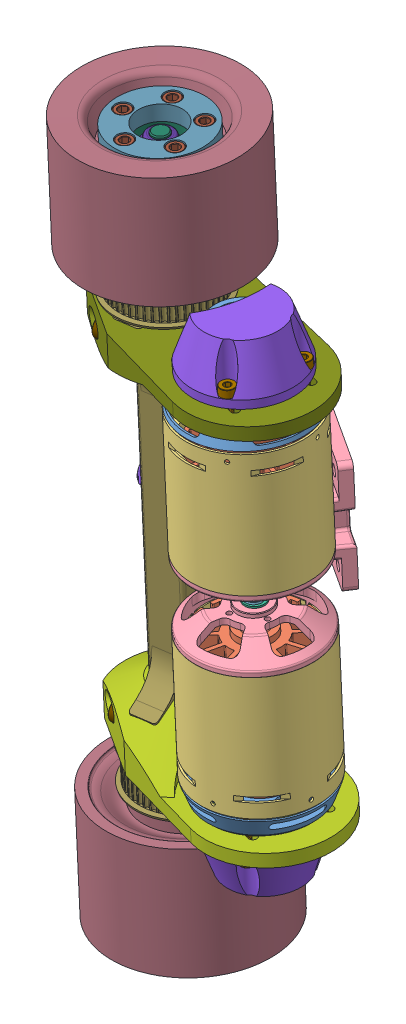
SolidWorks assembly MBS trucksV3, configuration Default. Lengths in mm.
Overall size (181.66 351.64 158.58).
89 component instances, 34 part files, 94 mates.
Components (placement in the parent):
- GPA26GT3150-A-N8-2: GPA26GT3150-A-N8 [Default] at (27.3667 -42.3784 -61.7275) x (-0.019038 0.999391 0.029249) z (0.735769 0.033812 -0.676388) size (20 28 28)
  - GPA26GT3150-A-N8_b-1: GPA26GT3150-A-N8_b [Default] at origin size (20 28 28)
  - SET-SCREW4-3-1: SET-SCREW4-3 [Default] at (10 5.4 0) x (0 -1 0) z (-1 0 0) size (3 4 4)
  - SET-SCREW4-3-2: SET-SCREW4-3 [Default] at (10 -2.2723 -3.2919) x (0 0.568065 0.822984) z (-1 0 0) size (3 4 4)
- Key20mm-2: Key20mm [Default] at (30.0951 -42.3485 -60.9758) x (-0.735769 -0.033812 0.676388) z (-0.676965 0.008644 -0.735964) size (3 20 3)
- MarkIITrucksCustomHangerV2-1: MarkIITrucksCustomHangerV2 [Default] at (-31.1638 36.2817 -181.4556) x (-0.019038 0.999391 0.029249) z (0.838104 0 0.54551) size (348 110.47 102.43)
  - 50cal_baseplateEDIT-1: 50cal_baseplateEDIT [Default] at (40.8754 28.4427 48.4148) size (55.88 41.6 78.53)
  - BS_bushing-1: BS_bushing [Default] at (40.8754 74.2758 55.8381) x (0.903515 -0.328294 -0.275471) z (-0.428557 -0.692132 -0.580768) size (24.64 14.73 24.64)
  - BS_washer-1: BS_washer [Default] at (40.8754 63.8267 68.2909) x (0.781233 0.478195 0.401253) z (-0.624239 0.59846 0.502167) size (29.08 4.06 29.08)
  - kingpin-1: kingpin [Default] at (40.8754 51.905 82.4986) x (0.057682 0.764769 0.641717) z (0.998335 -0.044187 -0.037077) size (16.06 70.1 13.91)
  - kingpin-nut-1: kingpin-nut [90630A115] at (40.8754 87.1097 40.5433) x (0.976709 0.16437 0.137923) z (-0.214569 0.748202 0.627816) size (12.7 8.97 14.66)
  - Pivot_cup-1: Pivot_cup [Default] at (40.8754 44.9216 26.2393) x (-0.987309 0.102082 -0.121656) z (0.158811 0.63463 -0.756323) size (17.46 19.05 17.46)
  - RS_bushing-1: RS_bushing [Default] at (40.8754 76.7422 52.8988) x (0.999722 0.018072 0.015164) z (-0.023591 0.765831 0.642609) size (24.77 14.61 24.77)
  - washer-1: washer [Default] at (171.3754 91.2507 63.4793) x (0 0.98686 -0.161575) z (0 0.161575 0.98686) size (11 1 11)
  - BS_washer-2: BS_washer [Default] at (40.8754 87.1097 40.5433) x (-0.947616 0.244683 0.205314) z (0.319411 0.725916 0.609116) size (29.08 4.06 29.08)
  - washer-2: washer [Default] at (196.6254 88.007 62.3923) x (0 -0.726217 0.687466) z (0 -0.687466 -0.726217) size (11 1 11)
  - CustomHangerV2-1: CustomHangerV2 [Default] at (40.8754 81.1126 56.6072) x (1 0 0) z (0 -0.642788 0.766044) size (260 93.96 18)
  - KegelWheelAssembly-1: KegelWheelAssembly [Default] at (208.2287 115.4342 118.578) x (0 0.174358 0.984682) z (0 -0.984682 0.174358) size (80 56 80)
    - Kegel 80mm longboard wheel-1: Kegel 80mm longboard wheel [Default] at (-60.1073 30.6906 17.2106) size (80 56 80)
    - 608-bearing-1: 608-bearing [6661K82] at (-60.1073 32.8534 17.2106) x (1 0 0) z (0 -1 0) size (22 22 7)
    - 608-bearing-2: 608-bearing [6661K82] at (-60.1073 15.6034 17.2106) x (-0.561464 0 0.827501) z (0 -1 0) size (22 22 7)
  - FPSSFJAD-D10-L100-T36-Q8-1: FPSSFJAD-D10-L100-T36-Q8 [Default] at (70.8754 88.007 62.3923) x (1 0 0) z (0 -0.599393 -0.800455) size (136 10 10)
  - SetScrew_SAE_10-32x.5in-1: SetScrew_SAE_10-32x.5in [92313A829] at (130.8754 96.8695 69.8289) x (0.758718 0.418725 -0.499016) z (0 0.766044 0.642788) size (4.96 4.83 13.07)
  - SetScrew_SAE_10-32x.5in-3: SetScrew_SAE_10-32x.5in [92313A829] at (130.8736 79.1457 54.9542) x (0.758718 0.418725 -0.499016) z (0 -0.766044 -0.642788) size (4.96 4.83 13.07)
  - NylonLockNut_5.16-24-1: NylonLockNut_5.16-24 [97135A225] at (197.1254 88.007 62.3923) x (0 0.323657 0.946174) z (0 0.946174 -0.323657) size (12.7 8.97 14.66)
  - KegelWheelAssembly-3: KegelWheelAssembly [Default] at (-126.478 81.5402 124.5797) x (0 0.174358 0.984682) z (0 0.984682 -0.174358) size (80 56 80)
    - Kegel 80mm longboard wheel-1: Kegel 80mm longboard wheel [Default] at (-60.1073 30.6906 17.2106) size (80 56 80)
    - 608-bearing-1: 608-bearing [6661K82] at (-60.1073 32.8534 17.2106) x (1 0 0) z (0 -1 0) size (22 22 7)
    - 608-bearing-2: 608-bearing [6661K82] at (-60.1073 15.6034 17.2106) x (-0.561464 0 0.827501) z (0 -1 0) size (22 22 7)
  - FPSSFJAD-D10-L100-T36-Q8-3: FPSSFJAD-D10-L100-T36-Q8 [Default] at (10.8754 88.007 62.3923) x (-1 0 0) z (0 0.599393 0.800455) size (136 10 10)
  - NylonLockNut_5.16-24-3: NylonLockNut_5.16-24 [97135A225] at (-115.3746 88.007 62.3923) x (0 -0.323657 -0.946174) z (0 0.946174 -0.323657) size (12.7 8.97 14.66)
  - SetScrew_SAE_10-32x.5in-7: SetScrew_SAE_10-32x.5in [92313A829] at (-49.1228 96.8708 69.8273) x (-0.758718 0.418725 -0.499016) z (0 0.766044 0.642788) size (4.96 4.83 13.07)
  - SetScrew_SAE_10-32x.5in-8: SetScrew_SAE_10-32x.5in [92313A829] at (-49.1246 79.1444 54.9557) x (-0.758718 0.418725 -0.499016) z (0 -0.766044 -0.642788) size (4.96 4.83 13.07)
- 91274A172_COATED ALLOY STEEL SOCKET HEAD CAP SCREW-1: 91274A172_COATED ALLOY STEEL SOCKET HEAD CAP SCREW [91274A172] at (-10.1778 -9.516 -60.2635) x (0.122495 -0.218247 0.968175) z (0.992459 0.022433 -0.12051) size (9.53 9.53 32.48)
- 91274A172_COATED ALLOY STEEL SOCKET HEAD CAP SCREW-2: 91274A172_COATED ALLOY STEEL SOCKET HEAD CAP SCREW [91274A172] at (-14.1739 -8.6338 -93.0088) x (-0.014856 -0.953854 -0.299902) z (0.992459 0.022433 -0.12051) size (9.53 9.53 32.48)
- 91274A172_COATED ALLOY STEEL SOCKET HEAD CAP SCREW-7: 91274A172_COATED ALLOY STEEL SOCKET HEAD CAP SCREW [91274A172] at (-13.3571 157.3822 -55.3789) x (-0.115179 -0.165774 -0.979414) z (0.992459 0.022433 -0.12051) size (9.53 9.53 32.48)
- Turnigy6374-6: Turnigy6374 [Default] at (19.4973 -4.0975 -58.6029) x (0.259506 0.033191 -0.965171) z (-0.965554 -0.010785 -0.25998) size (83.4 113.65 83.4)
  - Stator-1: Stator [Default] at (3.7873 1.8989 -6.3731) size (58.75 9.22 58.75)
  - StatorPart2-1: StatorPart2 [Default] at (3.7873 -16.3511 -6.3731) size (50 66 50)
  - AxelHoldCover-1: AxelHoldCover [Default] at (3.7873 -60.8511 -6.3731) x (0.982235 0 -0.187653) z (0.187653 0 0.982235) size (59.15 61.5 59.15)
  - AxelHold-1: AxelHold [Default] at (3.7873 -60.8511 -6.3731) x (0.729158 0 0.684345) z (0.684345 0 -0.729158) size (59 18.5 59)
  - AxisCust-1: AxisCust [Default] at (3.7873 -73.3511 -6.3731) x (0.844889 0 -0.534942) z (0.534942 0 0.844889) size (8 113.65 8)
  - 90967A120_STAINLESS STEEL EXTERNAL RETAINING RING-1: 90967A120_STAINLESS STEEL EXTERNAL RETAINING RING [90967A120] at (3.7873 12.2489 -6.3731) x (0 -1 0) z (0 0 1) size (0.8 12.1 9.85)
  - 90967A120_STAINLESS STEEL EXTERNAL RETAINING RING-2: 90967A120_STAINLESS STEEL EXTERNAL RETAINING RING [90967A120] at (3.7873 -73.7511 -6.3731) x (0 -1 0) z (-0.841191 0 -0.540738) size (0.8 12.1 9.85)
- MotorMountLeftV4-3: MotorMountLeftV4 [Default] at (-25.8025 -21.8807 -75.3183) x (-0.019038 0.999391 0.029249) z (-0.259506 -0.033191 0.965171) size (25.4 122.62 69.85)
- Belt Cap Wheel Side - Motor-2: Belt Cap Wheel Side - Motor [Default] at (26.965 -21.2913 -61.1104) x (-0.259506 -0.033191 0.965171) z (0.965554 0.010785 0.25998) size (50.8 25 40.64)
- M4x16mm_BlackZincSteel-3: M4x16mm_BlackZincSteel [91274A119] at (45.794 -8.6145 -71.7296) x (0.992084 0.022514 -0.123538) z (-0.019038 0.999391 0.029249) size (7 7 20.35)
- M4x16mm_BlackZincSteel-4: M4x16mm_BlackZincSteel [91274A119] at (37.7201 -9.6472 -41.7005) x (0.992084 0.022514 -0.123538) z (-0.019038 0.999391 0.029249) size (7 7 20.35)
- 92125A192_TYPE 18-8 SS FLAT-HEAD SOCKET CAP SCREW-9: 92125A192_TYPE 18-8 SS FLAT-HEAD SOCKET CAP SCREW [92125A192] at (15.9777 -20.7429 -80.1634) x (-0.507945 -0.034866 0.860683) z (0.019038 -0.999391 -0.029249) size (8 8 12.4)
- 92125A192_TYPE 18-8 SS FLAT-HEAD SOCKET CAP SCREW-10: 92125A192_TYPE 18-8 SS FLAT-HEAD SOCKET CAP SCREW [92125A192] at (7.9037 -21.7755 -50.1343) x (0.99191 0.022552 -0.124927) z (0.019038 -0.999391 -0.029249) size (8 8 12.4)
- 91251A355_BLACK-OXIDE ALLOY STEEL SOCKET HEAD CAP SCREW-11: 91251A355_BLACK-OXIDE ALLOY STEEL SOCKET HEAD CAP SCREW [91251A355] at (-41.267 -27.3016 -72.4744) x (0.999122 0.017925 0.037869) z (-0.019038 0.999391 0.029249) size (7.92 7.92 68.91)
- GPA50GT3150-A-H26_b-1: GPA50GT3150-A-H26_b [Default] at (-25.7787 -23.1299 -75.3548) x (0.019038 -0.999391 -0.029249) z (-0.18932 0.025122 -0.981594) size (20 51 51)
- Wheel Spacer 2-3: Wheel Spacer 2 [Default] at (-25.0284 -62.5187 -76.5076) x (-0.875178 -0.030803 0.482819) z (-0.483426 0.016407 -0.875231) size (44 14.02 44)
- Wheel Spacer Alum-3: Wheel Spacer Alum [Default] at (-25.0284 -62.5187 -76.5076) x (-0.875178 -0.030803 0.482819) z (-0.483426 0.016407 -0.875231) size (44 7.62 44)
- 91251A355_BLACK-OXIDE ALLOY STEEL SOCKET HEAD CAP SCREW-12: 91251A355_BLACK-OXIDE ALLOY STEEL SOCKET HEAD CAP SCREW [91251A355] at (-27.6611 -27.415 -59.7445) x (0.344241 0.034018 -0.938265) z (-0.019038 0.999391 0.029249) size (7.92 7.92 68.91)
- 91251A355_BLACK-OXIDE ALLOY STEEL SOCKET HEAD CAP SCREW-13: 91251A355_BLACK-OXIDE ALLOY STEEL SOCKET HEAD CAP SCREW [91251A355] at (-11.3541 -26.841 -68.7408) x (-0.786369 0.0031 -0.617749) z (-0.019038 0.999391 0.029249) size (7.92 7.92 68.91)
- 91251A355_BLACK-OXIDE ALLOY STEEL SOCKET HEAD CAP SCREW-14: 91251A355_BLACK-OXIDE ALLOY STEEL SOCKET HEAD CAP SCREW [91251A355] at (-14.8817 -26.3729 -87.0306) x (-0.830244 -0.032102 0.556475) z (-0.019038 0.999391 0.029249) size (7.92 7.92 68.91)
- 91251A355_BLACK-OXIDE ALLOY STEEL SOCKET HEAD CAP SCREW-15: 91251A355_BLACK-OXIDE ALLOY STEEL SOCKET HEAD CAP SCREW [91251A355] at (-33.3689 -26.6576 -89.3381) x (0.273251 -0.02294 0.961669) z (-0.019038 0.999391 0.029249) size (7.92 7.92 68.91)
- Wheel Spacer-3: Wheel Spacer [Default] at (-25.0284 -62.5187 -76.5076) x (-0.981731 -0.024225 0.188727) z (-0.18932 0.025122 -0.981594) size (44 7.02 44)
- 91274A172_COATED ALLOY STEEL SOCKET HEAD CAP SCREW-8: 91274A172_COATED ALLOY STEEL SOCKET HEAD CAP SCREW [91274A172] at (-13.3571 157.3822 -55.3789) x (-0.115179 -0.165774 -0.979414) z (0.992459 0.022433 -0.12051) size (9.53 9.53 32.48)
- 91274A172_COATED ALLOY STEEL SOCKET HEAD CAP SCREW-9: 91274A172_COATED ALLOY STEEL SOCKET HEAD CAP SCREW [91274A172] at (-17.3532 158.2645 -88.1242) x (0.051476 -0.968499 0.24364) z (0.992459 0.022433 -0.12051) size (9.53 9.53 32.48)
- Turnigy6374-7: Turnigy6374 [Default] at (28.8117 153.1465 -50.6911) x (0.259506 0.033191 -0.965171) z (0.965554 0.010785 0.25998) size (83.4 113.65 83.4)
  - Stator-1: Stator [Default] at (3.7873 1.8989 -6.3731) size (58.75 9.22 58.75)
  - StatorPart2-1: StatorPart2 [Default] at (3.7873 -16.3511 -6.3731) size (50 66 50)
  - AxelHoldCover-1: AxelHoldCover [Default] at (3.7873 -60.8511 -6.3731) x (0.982235 0 -0.187653) z (0.187653 0 0.982235) size (59.15 61.5 59.15)
  - AxelHold-1: AxelHold [Default] at (3.7873 -60.8511 -6.3731) x (0.729158 0 0.684345) z (0.684345 0 -0.729158) size (59 18.5 59)
  - AxisCust-1: AxisCust [Default] at (3.7873 -73.3511 -6.3731) x (0.844889 0 -0.534942) z (0.534942 0 0.844889) size (8 113.65 8)
  - 90967A120_STAINLESS STEEL EXTERNAL RETAINING RING-1: 90967A120_STAINLESS STEEL EXTERNAL RETAINING RING [90967A120] at (3.7873 12.2489 -6.3731) x (0 -1 0) z (0 0 1) size (0.8 12.1 9.85)
  - 90967A120_STAINLESS STEEL EXTERNAL RETAINING RING-2: 90967A120_STAINLESS STEEL EXTERNAL RETAINING RING [90967A120] at (3.7873 -73.7511 -6.3731) x (0 -1 0) z (-0.841191 0 -0.540738) size (0.8 12.1 9.85)
- Belt Cap Wheel Side - Motor-3: Belt Cap Wheel Side - Motor [Default] at (23.3097 170.5917 -55.4945) x (0.259506 0.033191 -0.965171) z (0.965554 0.010785 0.25998) size (50.8 25 40.64)
- M4x16mm_BlackZincSteel-5: M4x16mm_BlackZincSteel [91274A119] at (42.5956 159.2832 -66.8157) x (0.992084 0.022514 -0.123538) z (0.019038 -0.999391 -0.029249) size (7 7 20.35)
- M4x16mm_BlackZincSteel-6: M4x16mm_BlackZincSteel [91274A119] at (34.5217 158.2505 -36.7866) x (0.992084 0.022514 -0.123538) z (0.019038 -0.999391 -0.029249) size (7 7 20.35)
- 92125A192_TYPE 18-8 SS FLAT-HEAD SOCKET CAP SCREW-11: 92125A192_TYPE 18-8 SS FLAT-HEAD SOCKET CAP SCREW [92125A192] at (12.33 170.7404 -74.5592) x (0.507945 0.034866 -0.860683) z (-0.019038 0.999391 0.029249) size (8 8 12.4)
- 92125A192_TYPE 18-8 SS FLAT-HEAD SOCKET CAP SCREW-12: 92125A192_TYPE 18-8 SS FLAT-HEAD SOCKET CAP SCREW [92125A192] at (4.2561 169.7078 -44.5301) x (0.99191 0.022552 -0.124927) z (-0.019038 0.999391 0.029249) size (8 8 12.4)
- 91251A355_BLACK-OXIDE ALLOY STEEL SOCKET HEAD CAP SCREW-16: 91251A355_BLACK-OXIDE ALLOY STEEL SOCKET HEAD CAP SCREW [91251A355] at (-45.1142 174.6553 -66.5636) x (0.999122 0.017925 0.037869) z (0.019038 -0.999391 -0.029249) size (7.92 7.92 68.91)
- GPA50GT3150-A-H26_b-2: GPA50GT3150-A-H26_b [Default] at (-29.4816 171.2516 -69.6658) x (-0.019038 0.999391 0.029249) z (0.18932 -0.025122 0.981594) size (20 51 51)
- Wheel Spacer 2-4: Wheel Spacer 2 [Default] at (-30.2319 210.6404 -68.513) x (0.875178 0.030803 -0.482819) z (-0.483426 0.016407 -0.875231) size (44 14.02 44)
- Wheel Spacer Alum-4: Wheel Spacer Alum [Default] at (-30.2319 210.6404 -68.513) x (0.875178 0.030803 -0.482819) z (-0.483426 0.016407 -0.875231) size (44 7.62 44)
- Wheel Spacer-4: Wheel Spacer [Default] at (-30.2319 210.6404 -68.513) x (-0.981731 -0.024225 0.188727) z (0.18932 -0.025122 0.981594) size (44 7.02 44)
- GPA26GT3150-A-N8-3: GPA26GT3150-A-N8 [Default] at (23.2888 171.6911 -55.4623) x (-0.019038 0.999391 0.029249) z (0.735769 0.033812 -0.676388) size (20 28 28)
  - GPA26GT3150-A-N8_b-1: GPA26GT3150-A-N8_b [Default] at origin size (20 28 28)
  - SET-SCREW4-3-1: SET-SCREW4-3 [Default] at (10 5.4 0) x (0 -1 0) z (-1 0 0) size (3 4 4)
  - SET-SCREW4-3-2: SET-SCREW4-3 [Default] at (10 -2.2723 -3.2919) x (0 0.568065 0.822984) z (-1 0 0) size (3 4 4)
- Key20mm-3: Key20mm [Default] at (27.6673 191.6829 -51.9177) x (-0.735769 -0.033812 0.676388) z (0.676965 -0.008644 0.735964) size (3 20 3)
- MotorMountRightV4-2: MotorMountRightV4 [Default] at (-29.4578 170.0024 -69.7024) x (-0.019038 0.999391 0.029249) z (-0.259506 -0.033191 0.965171) size (25.4 122.62 69.85)
- 91251A355_BLACK-OXIDE ALLOY STEEL SOCKET HEAD CAP SCREW-17: 91251A355_BLACK-OXIDE ALLOY STEEL SOCKET HEAD CAP SCREW [91251A355] at (-37.2161 175.2993 -83.4274) x (-0.273251 0.02294 -0.961669) z (0.019038 -0.999391 -0.029249) size (7.92 7.92 68.91)
- 91251A355_BLACK-OXIDE ALLOY STEEL SOCKET HEAD CAP SCREW-18: 91251A355_BLACK-OXIDE ALLOY STEEL SOCKET HEAD CAP SCREW [91251A355] at (-18.7289 175.584 -81.1199) x (-0.830244 -0.032102 0.556475) z (0.019038 -0.999391 -0.029249) size (7.92 7.92 68.91)
- 91251A355_BLACK-OXIDE ALLOY STEEL SOCKET HEAD CAP SCREW-19: 91251A355_BLACK-OXIDE ALLOY STEEL SOCKET HEAD CAP SCREW [91251A355] at (-15.2013 175.1159 -62.8301) x (-0.786369 0.0031 -0.617749) z (0.019038 -0.999391 -0.029249) size (7.92 7.92 68.91)
- 91251A355_BLACK-OXIDE ALLOY STEEL SOCKET HEAD CAP SCREW-20: 91251A355_BLACK-OXIDE ALLOY STEEL SOCKET HEAD CAP SCREW [91251A355] at (-31.5083 174.5419 -53.8338) x (-0.344241 -0.034018 0.938265) z (0.019038 -0.999391 -0.029249) size (7.92 7.92 68.91)
Mates (geometry in assembly coordinates):
- Concentric1: concentric anti-aligned: cylinder of ? through (0 89.5 0) axis (0 -1 0) radius 6; cylinder of ? through (0 92.55 0) axis (0 1 0) radius 6
- Concentric2: concentric anti-aligned: cylinder of ? through (0 -26.5 0) axis (0 1 0) radius 4; cylinder of GPA26GT3150-A-N8-2/GPA26GT3150-A-N8_b-1 through (0 -6.5 0) axis (0 -1 0) radius 4
- Coincident1: coincident aligned: plane of ? through (0 -26.5 0) normal (0 -1 0); plane of GPA26GT3150-A-N8-2/GPA26GT3150-A-N8_b-1 through (0 -26.5 0) normal (0 -1 0)
- Coincident7: coincident anti-aligned: line of ? through (-1.5 -26.5 -2.5) axis (0 0 -1); line of GPA26GT3150-A-N8-2/GPA26GT3150-A-N8_b-1 through (-1.5 -26.5 -5.4) axis (0 0 1)
- Coincident8: coincident aligned: plane of GPA26GT3150-A-N8-2/GPA26GT3150-A-N8_b-1 through (27.3667 -42.3784 -61.7275) normal (0.019038 -0.999391 -0.029249); plane of Key20mm-2 through (30.0951 -42.3485 -60.9758) normal (0.019038 -0.999391 -0.029249)
- Coincident9: coincident anti-aligned: plane of ? through (1.5 -6.5 -2.5) normal (0 0 -1); plane of Key20mm-2 through (-1.5 -6.5 -2.5) normal (0 0 1)
- Coincident10: coincident anti-aligned: plane of GPA26GT3150-A-N8-2/GPA26GT3150-A-N8_b-1 through (31.7452 -22.3866 -58.1829) normal (-0.735769 -0.033812 0.676388); plane of Key20mm-2 through (29.7143 -22.3607 -60.3908) normal (0.735769 0.033812 -0.676388)
- Concentric5: concentric anti-aligned: cylinder of MarkIITrucksCustomHangerV2-1/CustomHangerV2-1 through (-77.4086 -5.45 -20.7444) axis (0 -1 0) radius 9; cylinder of ? through (-77.4086 -27.45 -20.7444) axis (0 1 0) radius 11
- Coincident15: coincident anti-aligned: plane of ? through (-77.2299 -26.5 -21.3999) normal (0 1 0); plane of ? through (-51.5162 -26.5 -25.2476) normal (0 -1 0)
- Coincident28: coincident anti-aligned: plane of MarkIITrucksCustomHangerV2-1/CustomHangerV2-1; plane of ? through (-34.0921 -14.7886 -63.0299) normal (-0.017088 0 -0.999854)
- Coincident37: coincident aligned: plane of ? through (-44.2534 59.243 -27.1128) normal (-0.40707 0 0.913397); plane of ? through (38.0802 32.893 9.5804) normal (-0.40707 0 0.913397)
- Coincident38: coincident anti-aligned: plane of ? through (-30.006 52.893 -59.0817) normal (0 -1 0); plane of ? through (52.3276 52.893 -22.3885) normal (0 1 0)
- Coincident40: coincident anti-aligned: plane of ? through (0 0 0) normal (0 -1 0); plane of ? through (-73.3266 0 -32.3363) normal (0 1 0)
- Concentric12: concentric aligned: cylinder of ? through (0 -26.5 0) axis (0 1 0) radius 4; cylinder of ? through (0 -6.35 0) axis (0 1 0) radius 6
- Coincident41: coincident anti-aligned: plane of ?; plane of ? through (-51.7284 -27.45 -24.8099) normal (0 -1 0)
- Concentric17: concentric aligned: cylinder of MarkIITrucksCustomHangerV2-1/CustomHangerV2-1 through (-34.2459 -20.2386 -72.0286) axis (0 -1 0) radius 9; cylinder of ? through (-34.2459 -22.2386 -72.0286) axis (0 -1 0) radius 10
- Coincident43: coincident anti-aligned: plane of ?; plane of ? through (-34.2459 -42.2386 -72.0286) normal (0 -1 0)
- Concentric18: concentric anti-aligned: cylinder of ? through (-93.4436 208.55 -19.2392) axis (0 -1 0) radius 2.54; cylinder of ? through (-93.4436 193.63 -19.2392) axis (0 1 0) radius 2.413
- Coincident45: coincident anti-aligned: plane of ? through (-93.4436 193.63 -19.2392) normal (0 -1 0); plane of ? through (-93.4436 193.63 -19.2392) normal (0 1 0)
- Concentric19: concentric: cylinder of ? through (-93.4436 208.55 -19.2392) axis (0 -1 0) radius 2.54; cylinder of ? through (-93.4436 193.63 -19.2392) axis (0 1 0) radius 2.413
- Coincident47: coincident anti-aligned: plane of ? through (-93.4436 193.63 -19.2392) normal (0 -1 0); plane of ? through (-93.4436 193.63 -19.2392) normal (0 1 0)
- Coincident48: coincident anti-aligned: plane of ? through (-29.8766 191.989 -69.0589) normal (0.019038 -0.999391 -0.029249); plane of ? through (-43.0816 192.3928 -91.4524) normal (-0.019038 0.999391 0.029249)
- Concentric28: concentric anti-aligned: cylinder of ? through (-15.3407 192.0809 -62.7407) axis (-0.019038 0.999391 0.029249) radius 2.9; cylinder of ? through (-16.2508 239.8547 -61.3425) axis (0.019038 -0.999391 -0.029249) radius 2.413
- Coincident56: coincident anti-aligned: plane of GPA26GT3150-A-N8-2/GPA26GT3150-A-N8_b-1 through (29.5379 -22.488 -56.1538) normal (-0.676965 0.008644 -0.735964); plane of Key20mm-2 through (31.7452 -22.3866 -58.1829) normal (0.676965 -0.008644 0.735964)
- Coincident58: coincident aligned: plane of GPA26GT3150-A-N8-2/GPA26GT3150-A-N8_b-1; plane of ? through (-22.9313 -22.2386 -48.6196) normal (0 1 0)
- Concentric38: concentric aligned: cylinder of MarkIITrucksCustomHangerV2-1/CustomHangerV2-1 through (-41.8828 -7.7386 -55.3957) axis (0.999854 0 -0.017088) radius 2.3813; cylinder of ? through (-80.4696 -7.7386 -54.7362) axis (0.999854 0 -0.017088) radius 5
- Concentric40: concentric aligned: cylinder of ? through (-81.0335 -7.7386 -87.7314) axis (0.999854 0 -0.017088) radius 5; cylinder of 91274A172_COATED ALLOY STEEL SOCKET HEAD CAP SCREW-2 through (-52.2253 -7.7386 -88.2237) axis (0.999854 0 -0.017088) radius 4.7625
- Concentric41: concentric aligned: cylinder of ? through (-80.4696 -7.7386 -54.7362) axis (0.999854 0 -0.017088) radius 5; cylinder of 91274A172_COATED ALLOY STEEL SOCKET HEAD CAP SCREW-1 through (-51.6614 -7.7386 -55.2286) axis (0.999854 0 -0.017088) radius 4.7625
- Coincident61: coincident anti-aligned: plane of ? through (-45.3123 -7.7386 -55.3371) normal (-0.999854 0 0.017088); plane of 91274A172_COATED ALLOY STEEL SOCKET HEAD CAP SCREW-1 through (-45.3123 -7.7386 -55.3371) normal (0.999854 0 -0.017088)
- Coincident62: coincident anti-aligned: plane of ? through (-45.8762 -7.7386 -88.3322) normal (-0.999854 0 0.017088); plane of 91274A172_COATED ALLOY STEEL SOCKET HEAD CAP SCREW-2 through (-45.8762 -7.7386 -88.3322) normal (0.999854 0 -0.017088)
- Coincident65: coincident anti-aligned: plane of MarkIITrucksCustomHangerV2-1/CustomHangerV2-1; plane of ? through (-40.595 4.2614 -71.9201) normal (0.999854 0 -0.017088)
- Coincident68: coincident anti-aligned: plane of ? through (-34.2459 -14.7886 -72.0286) normal (0 1 0); plane of Turnigy6374-6/Stator-1 through (52.6547 -14.7886 -33.3) normal (0 -1 0)
- Concentric46: concentric anti-aligned: cylinder of GPA26GT3150-A-N8-2/GPA26GT3150-A-N8_b-1 through (26.986 -22.3906 -61.1425) axis (0.019038 -0.999391 -0.029249) radius 4; cylinder of Turnigy6374-6/AxisCust-1 through (27.3505 -41.529 -61.7027) axis (-0.019038 0.999391 0.029249) radius 4
- Coincident70: coincident anti-aligned: plane of Key20mm-2 through (29.7143 -22.3607 -60.3908) normal (0.735769 0.033812 -0.676388); plane of Turnigy6374-6/AxisCust-1 through (31.8129 -22.3875 -58.1093) normal (-0.735769 -0.033812 0.676388)
- Concentric55: concentric aligned: cylinder of 91274A172_COATED ALLOY STEEL SOCKET HEAD CAP SCREW-1 through (-51.6614 -7.7386 -55.2286) axis (0.999854 0 -0.017088) radius 4.7625; cylinder of ? through (-80.4696 -7.7386 -54.7362) axis (0.999854 0 -0.017088) radius 3.175
- Coincident75: coincident anti-aligned: plane of 91274A172_COATED ALLOY STEEL SOCKET HEAD CAP SCREW-1; plane of ? through (-45.3123 -7.7386 -55.3371) normal (-0.999854 0 0.017088)
- Coincident76: coincident anti-aligned: plane of MarkIITrucksCustomHangerV2-1/CustomHangerV2-1; plane of ? through (-40.595 4.2614 -71.9201) normal (0.999854 0 -0.017088)
- Coincident77: coincident anti-aligned: plane of MarkIITrucksCustomHangerV2-1/CustomHangerV2-1; plane of ? through (-34.0921 -14.7886 -63.0299) normal (-0.017088 0 -0.999854)
- Concentric56: concentric aligned: cylinder of 91274A172_COATED ALLOY STEEL SOCKET HEAD CAP SCREW-2 through (-54.3819 -7.7386 -88.1869) axis (0.999854 0 -0.017088) radius 4.7625; cylinder of ? through (-81.0335 -7.7386 -87.7314) axis (0.999854 0 -0.017088) radius 5
- Concentric57: concentric aligned: cylinder of MarkIITrucksCustomHangerV2-1/CustomHangerV2-1 through (-41.8828 -7.7386 -55.3957) axis (0.999854 0 -0.017088) radius 2.3813; cylinder of ? through (-80.4696 -7.7386 -54.7362) axis (0.999854 0 -0.017088) radius 5
- Concentric58: concentric aligned: cylinder of 91274A172_COATED ALLOY STEEL SOCKET HEAD CAP SCREW-7 through (-51.6614 159.2614 -55.2286) axis (0.999854 0 -0.017088) radius 4.7625; cylinder of ? through (-80.4696 159.2614 -54.7362) axis (0.999854 0 -0.017088) radius 5
- Coincident78: coincident anti-aligned: plane of 91274A172_COATED ALLOY STEEL SOCKET HEAD CAP SCREW-7; plane of ? through (-45.3123 159.2614 -55.3371) normal (-0.999854 0 0.017088)
- Concentric59: concentric aligned: cylinder of 91274A172_COATED ALLOY STEEL SOCKET HEAD CAP SCREW-8 through (-52.2253 159.2614 -88.2237) axis (0.999854 0 -0.017088) radius 4.7625; cylinder of ? through (-81.0335 159.2614 -87.7314) axis (0.999854 0 -0.017088) radius 5
- Coincident79: coincident anti-aligned: plane of MarkIITrucksCustomHangerV2-1/CustomHangerV2-1; plane of ? through (-43.2446 -0.6886 -71.8748) normal (0.999854 0 -0.017088)
- Concentric60: concentric anti-aligned: cylinder of 91274A172_COATED ALLOY STEEL SOCKET HEAD CAP SCREW-2 through (-52.2253 -7.7386 -88.2237) axis (0.999854 0 -0.017088) radius 4.7625; circle of ?
- Coincident80: coincident anti-aligned: plane of 91274A172_COATED ALLOY STEEL SOCKET HEAD CAP SCREW-2; plane of ? through (-45.8762 -7.7386 -88.3322) normal (-0.999854 0 0.017088)
- Concentric61: concentric aligned: cylinder of MarkIITrucksCustomHangerV2-1/CustomHangerV2-1 through (-35.8988 -9.1248 -90.3708) axis (0.992459 0.022433 -0.12051) radius 2.3813; cylinder of 91274A172_COATED ALLOY STEEL SOCKET HEAD CAP SCREW-2 through (-45.6844 -9.346 -89.1826) axis (0.992459 0.022433 -0.12051) radius 4.7625
- Concentric62: concentric aligned: cylinder of MarkIITrucksCustomHangerV2-1/CustomHangerV2-1 through (-41.8828 -7.7386 -55.3957) axis (0.999854 0 -0.017088) radius 2.3813; cylinder of ? through (-80.4696 -7.7386 -54.7362) axis (0.999854 0 -0.017088) radius 3.175
- Concentric63: concentric: cylinder of 91274A172_COATED ALLOY STEEL SOCKET HEAD CAP SCREW-1 through (-51.6614 -7.7386 -55.2286) axis (0.999854 0 -0.017088) radius 4.7625; cylinder of ? through (-80.4696 -7.7386 -54.7362) axis (0.999854 0 -0.017088) radius 5
- Coincident81: coincident anti-aligned: plane of 91274A172_COATED ALLOY STEEL SOCKET HEAD CAP SCREW-1; plane of ? through (-45.3123 -7.7386 -55.3371) normal (-0.999854 0 0.017088)
- Coincident86: coincident aligned: plane of GPA26GT3150-A-N8-2/GPA26GT3150-A-N8_b-1 through (27.3667 -42.3784 -61.7275) normal (0.019038 -0.999391 -0.029249); plane of Turnigy6374-6/AxisCust-1 through (27.3667 -42.3784 -61.7275) normal (0.019038 -0.999391 -0.029249)
- Coincident87: coincident anti-aligned: plane of MarkIITrucksCustomHangerV2-1/CustomHangerV2-1; plane of ? through (-33.8358 147.2614 -48.0321) normal (-0.017088 0 -0.999854)
- Concentric72: concentric aligned: cylinder of MarkIITrucksCustomHangerV2-1/CustomHangerV2-1 through (-35.0821 156.8912 -52.7409) axis (0.992459 0.022433 -0.12051) radius 2.3813; cylinder of 91274A172_COATED ALLOY STEEL SOCKET HEAD CAP SCREW-7 through (-44.8677 156.67 -51.5527) axis (0.992459 0.022433 -0.12051) radius 4.7625
- Concentric73: concentric aligned: cylinder of 91274A172_COATED ALLOY STEEL SOCKET HEAD CAP SCREW-1 through (-41.6884 -10.2283 -56.4373) axis (0.992459 0.022433 -0.12051) radius 4.7625; cylinder of MotorMountLeftV4-3 through (-97.8787 -11.4984 -49.6144) axis (0.992459 0.022433 -0.12051) radius 5
- Concentric74: concentric aligned: cylinder of 91274A172_COATED ALLOY STEEL SOCKET HEAD CAP SCREW-2 through (-45.6844 -9.346 -89.1826) axis (0.992459 0.022433 -0.12051) radius 4.7625; cylinder of MotorMountLeftV4-3 through (-101.8748 -10.6161 -82.3596) axis (0.992459 0.022433 -0.12051) radius 5
- Coincident99: coincident anti-aligned: plane of MarkIITrucksCustomHangerV2-1/CustomHangerV2-1 through (-40.1271 204.0204 -76.5538) normal (-0.992459 -0.022433 0.12051); plane of MotorMountLeftV4-3 through (-34.8555 -15.7364 -74.0479) normal (0.992459 0.022433 -0.12051)
- Coincident100: coincident anti-aligned: plane of 91274A172_COATED ALLOY STEEL SOCKET HEAD CAP SCREW-1 through (-35.3862 -10.0858 -57.2026) normal (0.992459 0.022433 -0.12051); plane of MotorMountLeftV4-3 through (-35.3862 -10.0858 -57.2026) normal (-0.992459 -0.022433 0.12051)
- Coincident101: coincident anti-aligned: plane of 91274A172_COATED ALLOY STEEL SOCKET HEAD CAP SCREW-2 through (-39.3823 -9.2036 -89.9479) normal (0.992459 0.022433 -0.12051); plane of MotorMountLeftV4-3 through (-39.3823 -9.2036 -89.9479) normal (-0.992459 -0.022433 0.12051)
- Coincident108: coincident anti-aligned: plane of Turnigy6374-6/Stator-1 through (26.8441 -14.9452 -60.9246) normal (0.019038 -0.999391 -0.029249); plane of MotorMountLeftV4-3 through (-25.9234 -15.5345 -75.1325) normal (-0.019038 0.999391 0.029249)
- Concentric92: concentric aligned: cylinder of Belt Cap Wheel Side - Motor-2 through (46.5175 -46.5914 -72.8411) axis (-0.019038 0.999391 0.029249) radius 4; cylinder of M4x16mm_BlackZincSteel-3 through (46.1748 -28.6023 -72.3146) axis (-0.019038 0.999391 0.029249) radius 3.5
- Concentric93: concentric aligned: cylinder of Belt Cap Wheel Side - Motor-2 through (38.4435 -47.624 -42.812) axis (-0.019038 0.999391 0.029249) radius 4; cylinder of M4x16mm_BlackZincSteel-4 through (38.1008 -29.635 -42.2855) axis (-0.019038 0.999391 0.029249) radius 3.5
- Coincident121: coincident anti-aligned: plane of Belt Cap Wheel Side - Motor-2 through (46.0986 -24.6048 -72.1976) normal (0.019038 -0.999391 -0.029249); plane of M4x16mm_BlackZincSteel-3 through (46.0986 -24.6048 -72.1976) normal (-0.019038 0.999391 0.029249)
- Coincident122: coincident anti-aligned: plane of Belt Cap Wheel Side - Motor-2 through (38.0247 -25.6374 -42.1685) normal (0.019038 -0.999391 -0.029249); plane of M4x16mm_BlackZincSteel-4 through (38.0247 -25.6374 -42.1685) normal (-0.019038 0.999391 0.029249)
- Coincident123: coincident anti-aligned: plane of MotorMountLeftV4-3 through (-25.8025 -21.8807 -75.3183) normal (0.019038 -0.999391 -0.029249); plane of Belt Cap Wheel Side - Motor-2 through (26.965 -21.2913 -61.1104) normal (-0.019038 0.999391 0.029249)
- Tangent4: tangent anti-aligned: plane of MotorMountLeftV4-3; cone of ? through (71.8505 -7.1277 -46.5804) axis (-0.019038 0.999391 0.029249)
- Tangent5: tangent anti-aligned: plane of MotorMountLeftV4-3; cone of ? through (89.6321 -19.6632 -21.2486) axis (-0.019038 0.999391 0.029249)
- Tangent9: tangent anti-aligned: plane of MotorMountLeftV4-3; cone of ? through (89.6321 -19.6632 -21.2486) axis (-0.019038 0.999391 0.029249)
- Concentric105: concentric anti-aligned: cylinder of Turnigy6374-6/Stator-1 through (89.3833 -6.6015 -20.8663) axis (0.019038 -0.999391 -0.029249) radius 1.8559; circle of ?
- Concentric106: concentric anti-aligned: cylinder of Turnigy6374-6/Stator-1 through (71.8325 -6.1841 -46.5528) axis (0.019038 -0.999391 -0.029249) radius 1.8559; circle of ?
- Concentric107: concentric anti-aligned: cylinder of Turnigy6374-6/Stator-1 through (45.7261 -5.047 -71.6252) axis (0.019038 -0.999391 -0.029249) radius 1.8559; circle of M4x16mm_BlackZincSteel-3
- Concentric108: concentric anti-aligned: cylinder of Turnigy6374-6/Stator-1 through (37.6521 -6.0797 -41.5961) axis (0.019038 -0.999391 -0.029249) radius 1.8559; cylinder of M4x16mm_BlackZincSteel-4 through (38.1008 -29.635 -42.2855) axis (-0.019038 0.999391 0.029249) radius 3.5
- Tangent18: tangent anti-aligned: plane of MotorMountLeftV4-3 through (-20.5978 -21.215 -94.6761) normal (-0.170037 -0.730146 0.661796); cone of 92125A192_TYPE 18-8 SS FLAT-HEAD SOCKET CAP SCREW-9 through (15.9339 -18.4443 -80.0961) axis (-0.019038 0.999391 0.029249)
- Tangent19: tangent anti-aligned: plane of MotorMountLeftV4-3 through (-30.4061 -19.9649 -58.3003) normal (0.19696 -0.683206 -0.703161); cone of 92125A192_TYPE 18-8 SS FLAT-HEAD SOCKET CAP SCREW-10 through (7.86 -19.4769 -50.067) axis (-0.019038 0.999391 0.029249)
- Concentric109: concentric anti-aligned: cylinder of Turnigy6374-6/Stator-1 through (7.6111 -6.4152 -49.6848) axis (0.019038 -0.999391 -0.029249) radius 1.8559; circle of 92125A192_TYPE 18-8 SS FLAT-HEAD SOCKET CAP SCREW-10
- Concentric110: concentric anti-aligned: cylinder of Turnigy6374-6/Stator-1 through (15.6851 -5.3826 -79.7138) axis (0.019038 -0.999391 -0.029249) radius 1.8559; circle of 92125A192_TYPE 18-8 SS FLAT-HEAD SOCKET CAP SCREW-9
- Coincident124: coincident aligned: cone of MotorMountLeftV4-3 through (7.86 -19.4769 -50.067) axis (-0.019038 0.999391 0.029249); cone of 92125A192_TYPE 18-8 SS FLAT-HEAD SOCKET CAP SCREW-10 through (7.86 -19.4769 -50.067) axis (-0.019038 0.999391 0.029249)
- Coincident140: coincident anti-aligned: plane of ? through (-15.0116 238.8514 -69.4308) normal (0.019038 -0.999391 -0.029249); plane of ? through (-15.0116 238.8514 -69.4308) normal (-0.019038 0.999391 0.029249)
- Concentric122: concentric aligned: cylinder of MotorMountLeftV4-3 through (46.092 -24.255 -72.1873) axis (-0.019038 0.999391 0.029249) radius 2; cylinder of M4x16mm_BlackZincSteel-3 through (46.1748 -28.6023 -72.3146) axis (-0.019038 0.999391 0.029249) radius 3.5
- Concentric128: concentric anti-aligned: cylinder of 91251A355_BLACK-OXIDE ALLOY STEEL SOCKET HEAD CAP SCREW-11 through (-39.9662 -95.586 -74.4729) axis (-0.019038 0.999391 0.029249) radius 3.9624; cylinder of Wheel Spacer Alum-3 through (-40.0581 -90.7629 -74.3317) axis (0.019038 -0.999391 -0.029249) radius 3.9688
- Coincident145: coincident anti-aligned: plane of 91251A355_BLACK-OXIDE ALLOY STEEL SOCKET HEAD CAP SCREW-11 through (-40.0581 -90.7629 -74.3317) normal (-0.019038 0.999391 0.029249); plane of Wheel Spacer Alum-3 through (-40.0581 -90.7629 -74.3317) normal (0.019038 -0.999391 -0.029249)
- Coincident146: coincident aligned: circle of MarkIITrucksCustomHangerV2-1/KegelWheelAssembly-3/Kegel 80mm longboard wheel-1; circle of Wheel Spacer-3
- Concentric129: concentric aligned: cylinder of MarkIITrucksCustomHangerV2-1/KegelWheelAssembly-3/Kegel 80mm longboard wheel-1 through (-11.0312 -43.7907 -69.2369) axis (0.019038 -0.999391 -0.029249) radius 2.9; cylinder of Wheel Spacer-3 through (-10.3268 -80.7681 -70.3191) axis (0.019038 -0.999391 -0.029249) radius 2.54
- Coincident147: coincident anti-aligned: plane of Wheel Spacer Alum-3 through (-24.546 -87.8405 -77.2487) normal (-0.019038 0.999391 0.029249); plane of Wheel Spacer-3 through (-24.546 -87.8405 -77.2487) normal (0.019038 -0.999391 -0.029249)
- Concentric130: concentric aligned: circle of Wheel Spacer Alum-3; circle of Wheel Spacer-3
- Concentric131: concentric aligned: circle of Wheel Spacer Alum-3; circle of Wheel Spacer-3
- Concentric132: concentric aligned: cylinder of MarkIITrucksCustomHangerV2-1/KegelWheelAssembly-3/Kegel 80mm longboard wheel-1 through (-25.3837 -43.8673 -75.9618) axis (-0.019038 0.999391 0.029249) radius 40; cylinder of GPA50GT3150-A-H26_b-1 through (-25.3979 -43.1177 -75.9398) axis (-0.019038 0.999391 0.029249) radius 13
- Coincident148: coincident aligned: circle of MarkIITrucksCustomHangerV2-1/KegelWheelAssembly-3/Kegel 80mm longboard wheel-1; circle of Wheel Spacer 2-3
- Coincident149: coincident anti-aligned: plane of GPA50GT3150-A-H26_b-1 through (-46.0143 -43.6265 -71.9766) normal (0.019038 -0.999391 -0.029249); plane of Wheel Spacer 2-3 through (-25.3979 -43.1177 -75.9398) normal (-0.019038 0.999391 0.029249)
- Concentric133: concentric aligned: cylinder of Wheel Spacer 2-3 through (-27.086 -57.6066 -60.6282) axis (-0.019038 0.999391 0.029249) radius 2.54; cylinder of 91251A355_BLACK-OXIDE ALLOY STEEL SOCKET HEAD CAP SCREW-12 through (-26.4522 -90.8763 -61.6019) axis (-0.019038 0.999391 0.029249) radius 2.413
- Concentric134: concentric aligned: cylinder of GPA50GT3150-A-H26_b-1 through (-27.3525 -43.6151 -60.2187) axis (-0.019038 0.999391 0.029249) radius 2; cylinder of 91251A355_BLACK-OXIDE ALLOY STEEL SOCKET HEAD CAP SCREW-12 through (-26.4522 -90.8763 -61.6019) axis (-0.019038 0.999391 0.029249) radius 2.413
- Coincident150: coincident anti-aligned: plane of MarkIITrucksCustomHangerV2-1/CustomHangerV2-1 through (-35.0221 74.159 -80.6756) normal (-0.992459 -0.022433 0.12051); plane of MotorMountRightV4-2 through (-35.2763 144.4754 -69.6801) normal (0.992459 0.022433 -0.12051)
- Coincident151: coincident anti-aligned: plane of Turnigy6374-7/Stator-1 through (23.4306 164.2456 -55.6802) normal (-0.019038 0.999391 0.029249); plane of MotorMountRightV4-2 through (-29.3369 163.6562 -69.8881) normal (0.019038 -0.999391 -0.029249)
- Coincident152: coincident aligned: plane of MarkIITrucksCustomHangerV2-1/CustomHangerV2-1 through (-36.8498 170.1005 -77.8677) normal (-0.019038 0.999391 0.029249); plane of MotorMountRightV4-2 through (-29.4578 170.0024 -69.7024) normal (-0.019038 0.999391 0.029249)
- Coincident153: coincident anti-aligned: plane of MarkIITrucksCustomHangerV2-1/CustomHangerV2-1 through (-36.8385 74.56 -95.5598) normal (-0.121093 0.026735 -0.992281); plane of MotorMountRightV4-2 through (-31.8805 145.2595 -94.2601) normal (0.121093 -0.026735 0.992281)
